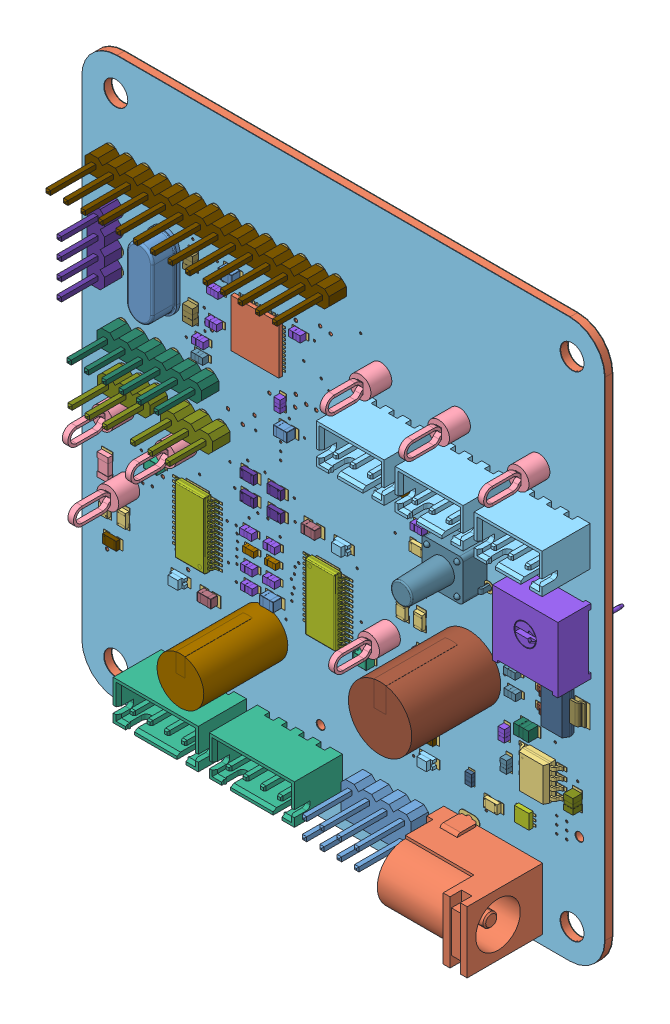
SolidWorks assembly PCBA_MAIN v1, configuration Default. Lengths in mm.
Overall size (76.2 81.28 25.69).
185 component instances, 42 part files, 0 mates.
Components (placement in the parent):
- PCBA_MAIN v1.step-1: PCBA_MAIN v1.step [Default] at origin size (76.2 81.28 25.69)
  - Packages.step-1: Packages.step [Default] at origin size (71.26 68.07 25.69)
    - CAPC2012X135N.step-1: CAPC2012X135N.step [Default] at (28.2191 24.238 1.1174) x (-1 0 0) z (0 0 1) size (2 1.35 1.25)
      - EMK212B7475KG-T v1.step-1: EMK212B7475KG-T v1.step [Default] at (0.053 -0.677 0.6501) size (2 1.35 1.25)
    - CUI_PJ-102AH.step-1: CUI_PJ-102AH.step [Default] at (60.0159 5.969 1.1174) size (14.4 9.4 14.5)
      - PJ-102AH v1.step-1: PJ-102AH v1.step [Default] at (7.1924 -0.0398 6.5417) x (1 0 0) z (0 -1 0) size (14.4 14.5 9.4)
    - RESC2012X60N.step-1: RESC2012X60N.step [Default] at (60.1144 14.3556 1.1174) size (2 1.25 0.6)
      - RC0805FR-0710KL v1.step-1: RC0805FR-0710KL v1.step [Default] at (0 -0.0013 0) x (1 0 0) z (0 -1 0) size (2 0.6 1.25)
    - RC1206N_YAG.step-1: RC1206N_YAG.step [Default] at (49.6142 27.1864 1.1174) x (0 1 0) z (0 0 1) size (3.2 1.6 0.71)
      - RC1206FR-071K5L v1.step-1: RC1206FR-071K5L v1.step [Default] at origin size (3.2 1.6 0.71)
    - B3B-XH-A.step-1: B3B-XH-A.step [Default] at (46.1225 53.8462 1.1174) size (9.9 5.75 10.4)
      - B3B-XH-A v1.step-1: B3B-XH-A v1.step [Default] x (1 0 0) z (0 -1 0) size (9.9 10.4 5.75)
        - BxB-XH-A_03.step-1: BxB-XH-A_03.step [Default] at (2.5 0 0.525) x (-1 0 0) z (0 0 -1) size (9.9 10.4 5.75)
    - B3B-XH-A.step-2: B3B-XH-A.step [Default] at (57.6291 53.8462 1.1174) size (9.9 5.75 10.4)
      - B3B-XH-A v1.step-1: B3B-XH-A v1.step [Default] x (1 0 0) z (0 -1 0) size (9.9 10.4 5.75)
        - BxB-XH-A_03.step-1: BxB-XH-A_03.step [Default] at (2.5 0 0.525) x (-1 0 0) z (0 0 -1) size (9.9 10.4 5.75)
    - B3B-XH-A.step-3: B3B-XH-A.step [Default] at (69.1356 53.8462 1.1174) size (9.9 5.75 10.4)
      - B3B-XH-A v1.step-1: B3B-XH-A v1.step [Default] x (1 0 0) z (0 -1 0) size (9.9 10.4 5.75)
        - BxB-XH-A_03.step-1: BxB-XH-A_03.step [Default] at (2.5 0 0.525) x (-1 0 0) z (0 0 -1) size (9.9 10.4 5.75)
    - B4B-XH-A.step-1: B4B-XH-A.step [Default] at (17.7825 6.6784 1.1174) size (12.4 5.75 10.4)
      - B4B-XH-A v1.step-1: B4B-XH-A v1.step [Default] x (1 0 0) z (0 -1 0.000058) size (12.4 10.4 5.75)
        - BxB-XH-A_04.step-1: BxB-XH-A_04.step [Default] at (3.75 0 0.525) x (-1 0 0) z (0 0 -1) size (12.4 10.4 5.75)
    - B4B-XH-A.step-2: B4B-XH-A.step [Default] at (31.789 6.6784 1.1174) size (12.4 5.75 10.4)
      - B4B-XH-A v1.step-1: B4B-XH-A v1.step [Default] x (1 0 0) z (0 -1 0.000058) size (12.4 10.4 5.75)
        - BxB-XH-A_04.step-1: BxB-XH-A_04.step [Default] at (3.75 0 0.525) x (-1 0 0) z (0 0 -1) size (12.4 10.4 5.75)
    - RC1206N_YAG.step-2: RC1206N_YAG.step [Default] at (3.7512 28.9814 1.1174) x (0 -1 0) z (0 0 1) size (3.2 1.6 0.71)
      - RC1206FR-071K5L v1.step-1: RC1206FR-071K5L v1.step [Default] at origin size (3.2 1.6 0.71)
    - IC_TPS61196PWPRQ1.step-1: IC_TPS61196PWPRQ1.step [Default] at (35.9029 27.9273 1.1174) size (6.4 9.7 1.2)
      - DRV8825 v1.step-1: DRV8825 v1.step [Default] at (0 0.0012 0.0023) x (1 0 0) z (0 -1 0) size (6.4 1.2 9.7)
    - IC_TPS61196PWPRQ1.step-2: IC_TPS61196PWPRQ1.step [Default] at (16.9037 28.1559 1.1174) x (-1 0 0) z (0 0 1) size (6.4 9.7 1.2)
      - DRV8825 v1.step-1: DRV8825 v1.step [Default] at (0 0.0012 0.0023) x (1 0 0) z (0 -1 0) size (6.4 1.2 9.7)
    - RESC2012X60N.step-2: RESC2012X60N.step [Default] at (49.5441 32.3812 1.1174) x (0 -1 0) z (0 0 1) size (2 1.25 0.6)
      - RC0805FR-0710KL v1.step-1: RC0805FR-0710KL v1.step [Default] at (0 -0.0013 0) x (1 0 0) z (0 -1 0) size (2 0.6 1.25)
    - YAG_CC0603_YAG.step-1: YAG_CC0603_YAG.step [Default] at (29.3564 49.7201 1.1174) x (0 1 0) z (0 0 1) size (1.7 0.91 0.91)
      - CC0603KRX7R8BB104 v1.step-1: CC0603KRX7R8BB104 v1.step [Default] at origin size (1.7 0.91 0.91)
    - YAG_CC0603_YAG.step-2: YAG_CC0603_YAG.step [Default] at (24.9036 24.2507 1.1174) size (1.7 0.91 0.91)
      - CC0603KRX7R8BB104 v1.step-1: CC0603KRX7R8BB104 v1.step [Default] at origin size (1.7 0.91 0.91)
    - YAG_CC0603_YAG.step-3: YAG_CC0603_YAG.step [Default] at (28.1823 31.115 1.1174) x (-1 0 0) z (0 0 1) size (1.7 0.91 0.91)
      - CC0603KRX7R8BB104 v1.step-1: CC0603KRX7R8BB104 v1.step [Default] at origin size (1.7 0.91 0.91)
    - YAG_CC0603_YAG.step-4: YAG_CC0603_YAG.step [Default] at (24.7767 31.1118 1.1174) size (1.7 0.91 0.91)
      - CC0603KRX7R8BB104 v1.step-1: CC0603KRX7R8BB104 v1.step [Default] at origin size (1.7 0.91 0.91)
    - RC0603N_PAN.step-1: RC0603N_PAN.step [Default] at (24.9555 28.8878 1.1174) x (-1 0 0) z (0 0 1) size (1.6 0.8 0.71)
      - ERJ-3EKF1004V v1.step-1: ERJ-3EKF1004V v1.step [Default] at origin size (1.6 0.8 0.71)
    - RC0603N_PAN.step-2: RC0603N_PAN.step [Default] at (28.1391 28.9386 1.1174) size (1.6 0.8 0.71)
      - ERJ-3EKF1004V v1.step-1: ERJ-3EKF1004V v1.step [Default] at origin size (1.6 0.8 0.71)
    - FUS_VISHAY_MFU0603_VIS.step-1: FUS_VISHAY_MFU0603_VIS.step [Default] at (56.8614 16.11 1.1174) x (0 1 0) z (0 0 1) size (1.6 1.02 0.64)
      - MFU0603FF04000P500 v1.step-1: MFU0603FF04000P500 v1.step [Default] at origin size (1.6 1.02 0.64)
    - YAG_CC0603_YAG.step-5: YAG_CC0603_YAG.step [Default] at (31.9012 59.7094 1.1174) x (-1 0 0) z (0 0 1) size (1.7 0.91 0.91)
      - CC0603KRX7R8BB104 v1.step-1: CC0603KRX7R8BB104 v1.step [Default] at origin size (1.7 0.91 0.91)
    - IND_BOURNS_RLB0914.step-1: IND_BOURNS_RLB0914.step [Default] at (56.4515 32.6898 1.1174) x (0 -1 0) z (0 0 1) size (9.24 9.22 17.52)
      - RLB0914_330KL v1.step-1: RLB0914_330KL v1.step [Default] at origin size (9.24 9.22 17.52)
    - RESC2012X60N.step-3: RESC2012X60N.step [Default] at (49.2916 41.275 1.1174) x (-1 0 0) z (0 0 1) size (2 1.25 0.6)
      - RC0805FR-0710KL v1.step-1: RC0805FR-0710KL v1.step [Default] at (0 -0.0013 0) x (1 0 0) z (0 -1 0) size (2 0.6 1.25)
    - YAG_CC0603_YAG.step-6: YAG_CC0603_YAG.step [Default] at (28.1364 26.746 1.1174) size (1.7 0.91 0.91)
      - CC0603KRX7R8BB104 v1.step-1: CC0603KRX7R8BB104 v1.step [Default] at origin size (1.7 0.91 0.91)
    - YAG_CC0603_YAG.step-7: YAG_CC0603_YAG.step [Default] at (49.6033 44.2214 1.1174) size (1.7 0.91 0.91)
      - CC0603KRX7R8BB104 v1.step-1: CC0603KRX7R8BB104 v1.step [Default] at origin size (1.7 0.91 0.91)
    - YAG_CC0603_YAG.step-8: YAG_CC0603_YAG.step [Default] at (24.8956 26.6764 1.1174) x (-1 0 0) z (0 0 1) size (1.7 0.91 0.91)
      - CC0603KRX7R8BB104 v1.step-1: CC0603KRX7R8BB104 v1.step [Default] at origin size (1.7 0.91 0.91)
    - YAG_CC0603_YAG.step-9: YAG_CC0603_YAG.step [Default] at (62.0416 24.4877 1.1174) x (0 -1 0) z (0 0 1) size (1.7 0.91 0.91)
      - CC0603KRX7R8BB104 v1.step-1: CC0603KRX7R8BB104 v1.step [Default] at origin size (1.7 0.91 0.91)
    - YAG_CC0603_YAG.step-10: YAG_CC0603_YAG.step [Default] at (19.7274 55.0224 1.1174) size (1.7 0.91 0.91)
      - CC0603KRX7R8BB104 v1.step-1: CC0603KRX7R8BB104 v1.step [Default] at origin size (1.7 0.91 0.91)
    - YAG_CC0603_YAG.step-11: YAG_CC0603_YAG.step [Default] at (19.91 59.2134 1.1174) size (1.7 0.91 0.91)
      - CC0603KRX7R8BB104 v1.step-1: CC0603KRX7R8BB104 v1.step [Default] at origin size (1.7 0.91 0.91)
    - RESC2012X60N.step-4: RESC2012X60N.step [Default] at (62.8142 40.9448 1.1174) x (0 1 0) z (0 0 1) size (2 1.25 0.6)
      - RC0805FR-0710KL v1.step-1: RC0805FR-0710KL v1.step [Default] at (0 -0.0013 0) x (1 0 0) z (0 -1 0) size (2 0.6 1.25)
    - RESC2012X60N.step-5: RESC2012X60N.step [Default] at (3.6741 23.6889 1.1174) x (0 1 0) z (0 0 1) size (2 1.25 0.6)
      - RC0805FR-0710KL v1.step-1: RC0805FR-0710KL v1.step [Default] at (0 -0.0013 0) x (1 0 0) z (0 -1 0) size (2 0.6 1.25)
    - RESC2012X60N.step-6: RESC2012X60N.step [Default] at (6.3335 23.6818 1.1174) x (0 -1 0) z (0 0 1) size (2 1.25 0.6)
      - RC0805FR-0710KL v1.step-1: RC0805FR-0710KL v1.step [Default] at (0 -0.0013 0) x (1 0 0) z (0 -1 0) size (2 0.6 1.25)
    - RESC2012X60N.step-7: RESC2012X60N.step [Default] at (47.0521 32.3676 1.1174) x (0 1 0) z (0 0 1) size (2 1.25 0.6)
      - RC0805FR-0710KL v1.step-1: RC0805FR-0710KL v1.step [Default] at (0 -0.0013 0) x (1 0 0) z (0 -1 0) size (2 0.6 1.25)
    - CAPC220145_88N_KEM.step-1: CAPC220145_88N_KEM.step [Default] at (16.2827 61.1915 1.1174) x (0 -1 0) z (0 0 1) size (2.2 1.45 0.88)
      - CAPC220145_88N_KEM v1.step-1: CAPC220145_88N_KEM v1.step [Default] at origin size (2.2 1.45 0.88)
    - CAPC220145_88N_KEM.step-2: CAPC220145_88N_KEM.step [Default] at (16.278 54.5563 1.1174) x (0 1 0) z (0 0 1) size (2.2 1.45 0.88)
      - CAPC220145_88N_KEM v1.step-1: CAPC220145_88N_KEM v1.step [Default] at origin size (2.2 1.45 0.88)
    - CAPC2012X100N.step-1: CAPC2012X100N.step [Default] at (18.7833 19.8409 1.1174) size (2 1.25 1)
      - C0805X103J1GECAUTO v1.step-1: C0805X103J1GECAUTO v1.step [Default] at (0.015 0.0165 0) x (1 0 0) z (0 -1 0) size (2 1 1.25)
    - CAPC2012X100N_1.step-1: CAPC2012X100N_1.step [Default] at (33.9327 36.0947 1.1174) x (-1 0 0) z (0 0 1) size (2 1.25 1)
      - C0805X103J1GECAUTO v1.step-1: C0805X103J1GECAUTO v1.step [Default] at (0.015 0.0165 0) x (1 0 0) z (0 -1 0) size (2 1 1.25)
    - YAG_CC0603_YAG (1).step-1: YAG_CC0603_YAG (1).step [Default] at (62.3422 20.701 1.1174) x (0 1 0) z (0 0 1) size (1.7 0.91 0.91)
      - CC0603KRX5R8BB105 v1.step-1: CC0603KRX5R8BB105 v1.step [Default] at origin size (1.7 0.91 0.91)
    - CAP_CC0805_YAG.step-1: CAP_CC0805_YAG.step [Default] at (65.4382 26.7144 1.1174) size (2.2 1.45 1.45)
      - CC0805MKX5R8BB226 v1.step-1: CC0805MKX5R8BB226 v1.step [Default] at origin size (2.2 1.45 1.45)
    - CAPC2012X135N (1).step-1: CAPC2012X135N (1).step [Default] at (72.2588 21.0237 1.1174) x (0 1 0) z (0 0 1) size (2.11 1.39 1.39)
      - EMK212BJ106KG-T v1.step-1: EMK212BJ106KG-T v1.step [Default] at origin size (2.11 1.39 1.39)
    - RESC2012X65N.step-1: RESC2012X65N.step [Default] at (28.6341 38.2651 1.1174) size (2 1.25 0.65)
      - ERJ-U6SFR20V v1.step-1: ERJ-U6SFR20V v1.step [Default] at (0 0.0142 0.0031) x (1 0 0) z (0 -1 0) size (2 0.65 1.25)
    - RESC2012X65N_1.step-1: RESC2012X65N_1.step [Default] at (28.6341 35.3568 1.1174) size (2 1.25 0.65)
      - ERJ-U6SFR20V v1.step-1: ERJ-U6SFR20V v1.step [Default] at (0 0.0142 0.0031) x (1 0 0) z (0 -1 0) size (2 0.65 1.25)
    - RESC2012X65N_2.step-1: RESC2012X65N_2.step [Default] at (24.687 35.3568 1.1174) x (-1 0 0) z (0 0 1) size (2 1.25 0.65)
      - ERJ-U6SFR20V v1.step-1: ERJ-U6SFR20V v1.step [Default] at (0 0.0142 0.0031) x (1 0 0) z (0 -1 0) size (2 0.65 1.25)
    - RESC2012X65N_3.step-1: RESC2012X65N_3.step [Default] at (24.687 38.2651 1.1174) x (-1 0 0) z (0 0 1) size (2 1.25 0.65)
      - ERJ-U6SFR20V v1.step-1: ERJ-U6SFR20V v1.step [Default] at (0 0.0142 0.0031) x (1 0 0) z (0 -1 0) size (2 0.65 1.25)
    - RESC2012X60N (1).step-1: RESC2012X60N (1).step [Default] at (47.7922 47.4726 1.1174) size (2 1.25 0.6)
      - RC0805FR-071KL v1.step-1: RC0805FR-071KL v1.step [Default] at (0 0.025 -0.0002) x (1 0 0) z (0 -1 0) size (2 0.6 1.25)
    - XTAL_HC49P488W43L1085T450H368.step-1: XTAL_HC49P488W43L1085T450H368.step [Default] at (12.0777 57.8358 1.1174) x (0 -1 0) z (0 0 1) size (10.85 4.5 16.38)
      - ATS08A-E v1.step-1: ATS08A-E v1.step [Default] at (0 0.0009 0.0079) x (1 0 0) z (0 -1 0.000073) size (10.85 16.38 4.5)
    - STM32F411CEU6.step-1: STM32F411CEU6.step [Default] at (25.8324 56.4642 1.1174) size (7 7 0.6)
      - STM32F411CEU6 v1.step-1: STM32F411CEU6 v1.step [Default] at (0 0.008 0.0102) x (1 0 0) z (0 -1 0) size (7 0.6 7)
    - SO8L_L6981N33DR_STM.step-1: SO8L_L6981N33DR_STM.step [Default] at (67.256 22.0345 1.1174) size (6.2 5.01 1.76)
      - L6981N50DR v1.step-1: L6981N50DR v1.step [Default] at origin size (6.2 5.01 1.76)
    - CAPC2012X135N_1.step-1: CAPC2012X135N_1.step [Default] at (30.2227 46.6794 1.1174) x (-1 0 0) z (0 0 1) size (2 1.35 1.25)
      - EMK212B7475KG-T v1.step-1: EMK212B7475KG-T v1.step [Default] at (0.053 -0.677 0.6501) size (2 1.35 1.25)
    - TP_5127.step-1: TP_5127.step [Default] at (6.0723 37.5069 1.1174) x (0 1 0) z (0 0 1) size (3.17 3.17 11.42)
      - 5127 v1.step-1: 5127 v1.step [Default] at (-0.143 0.2466 2.0375) x (1 0 0) z (0 -1 0) size (3.17 11.42 3.17)
    - TP_5127_1.step-1: TP_5127_1.step [Default] at (6.8805 27.8549 1.1174) x (0 1 0) z (0 0 1) size (3.17 3.17 11.42)
      - 5127 v1.step-1: 5127 v1.step [Default] at (-0.143 0.2466 2.0375) x (1 0 0) z (0 -1 0) size (3.17 11.42 3.17)
    - TP_5127_2.step-1: TP_5127_2.step [Default] at (15.2394 37.5069 1.1174) x (0 1 0) z (0 0 1) size (3.17 3.17 11.42)
      - 5127 v1.step-1: 5127 v1.step [Default] at (-0.143 0.2466 2.0375) x (1 0 0) z (0 -1 0) size (3.17 11.42 3.17)
    - TP_5127_3.step-1: TP_5127_3.step [Default] at (44.8766 28.2359 1.1174) x (0 1 0) z (0 0 1) size (3.17 3.17 11.42)
      - 5127 v1.step-1: 5127 v1.step [Default] at (-0.143 0.2466 2.0375) x (1 0 0) z (0 -1 0) size (3.17 11.42 3.17)
    - TP_5127_4.step-1: TP_5127_4.step [Default] at (43.6297 60.2399 1.1174) x (0 1 0) z (0 0 1) size (3.17 3.17 11.42)
      - 5127 v1.step-1: 5127 v1.step [Default] at (-0.143 0.2466 2.0375) x (1 0 0) z (0 -1 0) size (3.17 11.42 3.17)
    - TP_5127_5.step-1: TP_5127_5.step [Default] at (55.0829 60.2399 1.1174) x (0 1 0) z (0 0 1) size (3.17 3.17 11.42)
      - 5127 v1.step-1: 5127 v1.step [Default] at (-0.143 0.2466 2.0375) x (1 0 0) z (0 -1 0) size (3.17 11.42 3.17)
    - TP_5127_6.step-1: TP_5127_6.step [Default] at (66.663 60.2399 1.1174) x (0 1 0) z (0 0 1) size (3.17 3.17 11.42)
      - 5127 v1.step-1: 5127 v1.step [Default] at (-0.143 0.2466 2.0375) x (1 0 0) z (0 -1 0) size (3.17 11.42 3.17)
    - RESC2012X60N (1).step-2: RESC2012X60N (1).step [Default] at (45.4586 18.288 1.1174) x (-1 0 0) z (0 0 1) size (2 1.25 0.6)
      - RC0805FR-071KL v1.step-1: RC0805FR-071KL v1.step [Default] at (0 0.025 -0.0002) x (1 0 0) z (0 -1 0) size (2 0.6 1.25)
    - RESC2012X60N (1).step-3: RESC2012X60N (1).step [Default] at (50.7492 18.3134 1.1174) x (-1 0 0) z (0 0 1) size (2 1.25 0.6)
      - RC0805FR-071KL v1.step-1: RC0805FR-071KL v1.step [Default] at (0 0.025 -0.0002) x (1 0 0) z (0 -1 0) size (2 0.6 1.25)
    - LED_VCCLITE_0805_VCC.step-1: LED_VCCLITE_0805_VCC.step [Default] at (44.1452 47.4387 1.1174) size (2 1.25 1.2)
      - VAOL-S8SB4 v1.step-1: VAOL-S8SB4 v1.step [Default] x (1 0 0) z (0 -1 0) size (2 1.2 1.25)
        - CMD17xxx_Green.step-1: CMD17xxx_Green.step [Default] at origin size (2 1.2 1.25)
    - LED_VCCLITE_0805_VCC.step-2: LED_VCCLITE_0805_VCC.step [Default] at (45.339 15.3162 1.1174) size (2 1.25 1.2)
      - VAOL-S8SB4 v1.step-1: VAOL-S8SB4 v1.step [Default] x (1 0 0) z (0 -1 0) size (2 1.2 1.25)
        - CMD17xxx_Green.step-1: CMD17xxx_Green.step [Default] at origin size (2 1.2 1.25)
    - LED_VCCLITE_0805_VCC.step-3: LED_VCCLITE_0805_VCC.step [Default] at (50.7238 15.2654 1.1174) size (2 1.25 1.2)
      - VAOL-S8SB4 v1.step-1: VAOL-S8SB4 v1.step [Default] x (1 0 0) z (0 -1 0) size (2 1.2 1.25)
        - CMD17xxx_Green.step-1: CMD17xxx_Green.step [Default] at origin size (2 1.2 1.25)
    - RESC2012X60N (1).step-4: RESC2012X60N (1).step [Default] at (4.6139 19.9023 1.1174) x (-1 0 0) z (0 0 1) size (2 1.25 0.6)
      - RC0805FR-071KL v1.step-1: RC0805FR-071KL v1.step [Default] at (0 0.025 -0.0002) x (1 0 0) z (0 -1 0) size (2 0.6 1.25)
    - RESC2012X60N (1).step-5: RESC2012X60N (1).step [Default] at (48.8275 36.0591 1.1174) size (2 1.25 0.6)
      - RC0805FR-071KL v1.step-1: RC0805FR-071KL v1.step [Default] at (0 0.025 -0.0002) x (1 0 0) z (0 -1 0) size (2 0.6 1.25)
    - LED_VCCLITE_0805_VCC.step-4: LED_VCCLITE_0805_VCC.step [Default] at (14.4907 20.0343 1.1174) x (-1 0 0) z (0 0 1) size (2 1.25 1.2)
      - VAOL-S8SB4 v1.step-1: VAOL-S8SB4 v1.step [Default] x (1 0 0) z (0 -1 0) size (2 1.2 1.25)
        - CMD17xxx_Green.step-1: CMD17xxx_Green.step [Default] at origin size (2 1.2 1.25)
    - LED_VCCLITE_0805_VCC.step-5: LED_VCCLITE_0805_VCC.step [Default] at (38.2905 36.0934 1.1174) size (2 1.25 1.2)
      - VAOL-S8SB4 v1.step-1: VAOL-S8SB4 v1.step [Default] x (1 0 0) z (0 -1 0) size (2 1.2 1.25)
        - CMD17xxx_Green.step-1: CMD17xxx_Green.step [Default] at origin size (2 1.2 1.25)
    - CAP_CGJ4J2X7R0J474K125AA.step-1: CAP_CGJ4J2X7R0J474K125AA.step [Default] at (11.176 33.1216 1.1174) x (-1 0 0) z (0 0 1) size (2 1.45 1.25)
      - CGJ4J2X7R0J474K125AA v1.step-1: CGJ4J2X7R0J474K125AA v1.step [Default] at (0 -0.7 0.6) size (2 1.45 1.25)
    - CAP_CGJ4J2X7R0J474K125AA.step-2: CAP_CGJ4J2X7R0J474K125AA.step [Default] at (41.6814 23.6982 1.1174) size (2 1.45 1.25)
      - CGJ4J2X7R0J474K125AA v1.step-1: CGJ4J2X7R0J474K125AA v1.step [Default] at (0 -0.7 0.6) size (2 1.45 1.25)
    - DFN2020MD-6_SOT1220_NEX.step-1: DFN2020MD-6_SOT1220_NEX.step [Default] at (64.77 15.24 1.1174) size (2.11 2.11 0.66)
      - DFN2020MD-6_SOT1220_NEX v1.step-1: DFN2020MD-6_SOT1220_NEX v1.step [Default] at origin size (2.11 2.11 0.66)
    - POT_3386P.step-1: POT_3386P.step [Default] at (66.9036 41.91 1.1174) size (9.53 9.53 11.68)
      - 3386P-1-502LF v1.step-1: 3386P-1-502LF v1.step [Default] at (2.5438 0.02 0.0026) x (1 0 0) z (0 -1 0) size (9.53 11.68 9.53)
    - CAP_WCAP-ATG5_6.3X11_WRE.step-1: CAP_WCAP-ATG5_6.3X11_WRE.step [Default] at (26.6192 17.9832 1.1174) x (0 1 0) z (0 0 1) size (6.84 6.81 16.47)
      - CAP_WCAP-ATG5_6_3x11_WRE v1.step-1: CAP_WCAP-ATG5_6_3x11_WRE v1.step [Default] at origin size (6.84 6.81 16.47)
    - YAG_CC0603_YAG (1).step-2: YAG_CC0603_YAG (1).step [Default] at (63.2829 30.1438 1.1174) size (1.7 0.91 0.91)
      - CC0603KRX5R8BB105 v1.step-1: CC0603KRX5R8BB105 v1.step [Default] at origin size (1.7 0.91 0.91)
    - YAG_CC0603_YAG (1).step-3: YAG_CC0603_YAG (1).step [Default] at (63.2206 32.8168 1.1174) size (1.7 0.91 0.91)
      - CC0603KRX5R8BB105 v1.step-1: CC0603KRX5R8BB105 v1.step [Default] at origin size (1.7 0.91 0.91)
    - VREG_TLV1117LV33DCYR.step-1: VREG_TLV1117LV33DCYR.step [Default] at (70.1294 32.3215 1.1174) size (7 6.5 1.68)
      - DCY0004A v1.step-1: DCY0004A v1.step [Default] at origin size (7 6.5 1.68)
        - BODY-SOT.step-1: BODY-SOT.step [Default] at (0 0 0.7874) x (0 -1 0) z (-1 0 0) size (6.5 1.6 3.5)
        - LEAD-SOT.step-1: LEAD-SOT.step [Default] at (-2.7498 -2.2438 0.25) x (0 -1 0) z (-1 0 0) size (0.75 0.79 1.75)
        - LEAD-SOT.step-2: LEAD-SOT.step [Default] at (-2.7498 0.0562 0.25) x (0 -1 0) z (-1 0 0) size (0.75 0.79 1.75)
        - LEAD-SOT.step-3: LEAD-SOT.step [Default] at (-2.7498 2.3562 0.25) x (0 -1 0) z (-1 0 0) size (0.75 0.79 1.75)
        - LEAD-SOT-WIDE.step-1: LEAD-SOT-WIDE.step [Default] at (2.7498 0.0026 0.25) x (0 1 0) z (1 0 0) size (3 0.79 1.75)
    - SW_TL1105BF160Q.step-1: SW_TL1105BF160Q.step [Default] at (56.0578 43.561 1.1174) size (7.89 6 13.05)
      - TL1105BF160Q v1.step-1: TL1105BF160Q v1.step [Default] x (1 0 0) z (0 -1 0) size (7.89 13.05 6)
        - TL1105BF160Q--3DModel-STEP-520916.STEP.step-1: TL1105BF160Q--3DModel-STEP-520916.STEP.step [Default] at (0 1.79 0) x (1 0 0) z (0 1 0) size (7.89 6 13.05)
          - Body1.STEP.step-1: Body1.STEP.step [Default] at origin size (5.02 5.02 0.32)
          - Body2.STEP.step-1: Body2.STEP.step [Default] at origin size (7.89 6 13.05)
    - CAPC2012X135N_2.step-1: CAPC2012X135N_2.step [Default] at (22.098 62.484 1.1174) size (2 1.35 1.25)
      - EMK212B7475KG-T v1.step-1: EMK212B7475KG-T v1.step [Default] at (0 -0.677 0.6501) size (2 1.35 1.25)
    - YAG_CC0603_YAG (1).step-4: YAG_CC0603_YAG (1).step [Default] at (17.6784 49.784 1.1174) size (1.7 0.91 0.91)
      - CC0603KRX5R8BB105 v1.step-1: CC0603KRX5R8BB105 v1.step [Default] at origin size (1.7 0.91 0.91)
    - YAG_CC0603_YAG.step-12: YAG_CC0603_YAG.step [Default] at (17.7546 51.7906 1.1174) size (1.7 0.91 0.91)
      - CC0603KRX7R8BB104 v1.step-1: CC0603KRX7R8BB104 v1.step [Default] at origin size (1.7 0.91 0.91)
    - 1X06.step-1: 1X06.step [Default] at (12.3444 47.0501 1.1174) x (-1 0 0) z (0 0 1) size (15.24 2.54 11.34)
    - 1X03.step-1: 1X03.step [Default] at (17.8054 41.4113 1.1174) size (7.62 2.54 11.34)
    - 1X03.step-2: 1X03.step [Default] at (8.6614 41.4113 1.1174) size (7.62 2.54 11.34)
    - 1X04.step-1: 1X04.step [Default] at (4.5627 58.1406 1.1174) x (0 -1 0) z (0 0 1) size (10.16 2.54 11.34)
    - 1X14.step-1: 1X14.step [Default] at (20.7772 68.2463 1.1174) x (-1 0 0) z (0 0 1) size (35.56 2.54 12.64)
    - 2X04.step-1: 2X04.step [Default] at (45.4152 6.6111 1.1174) x (-1 0 0) z (0 0 1) size (10.16 5.08 12.64)
  - Board.step-1: Board.step [Default] at origin size (76.2 81.28 1.04)
  - 1-copper.step-1: 1-copper.step [Default] at (0 0 1.037) size (74.05 79.1 0.13)
  - 16-copper.step-1: 16-copper.step [Default] at (0 0 -0.035) size (74.05 79.1 0.13)
  - 1-soldermask.step-1: 1-soldermask.step [Default] at (0 0 1.037) size (76.2 81.28 0.08)
  - 16-soldermask.step-1: 16-soldermask.step [Default] at origin size (76.2 81.28 0.08)
